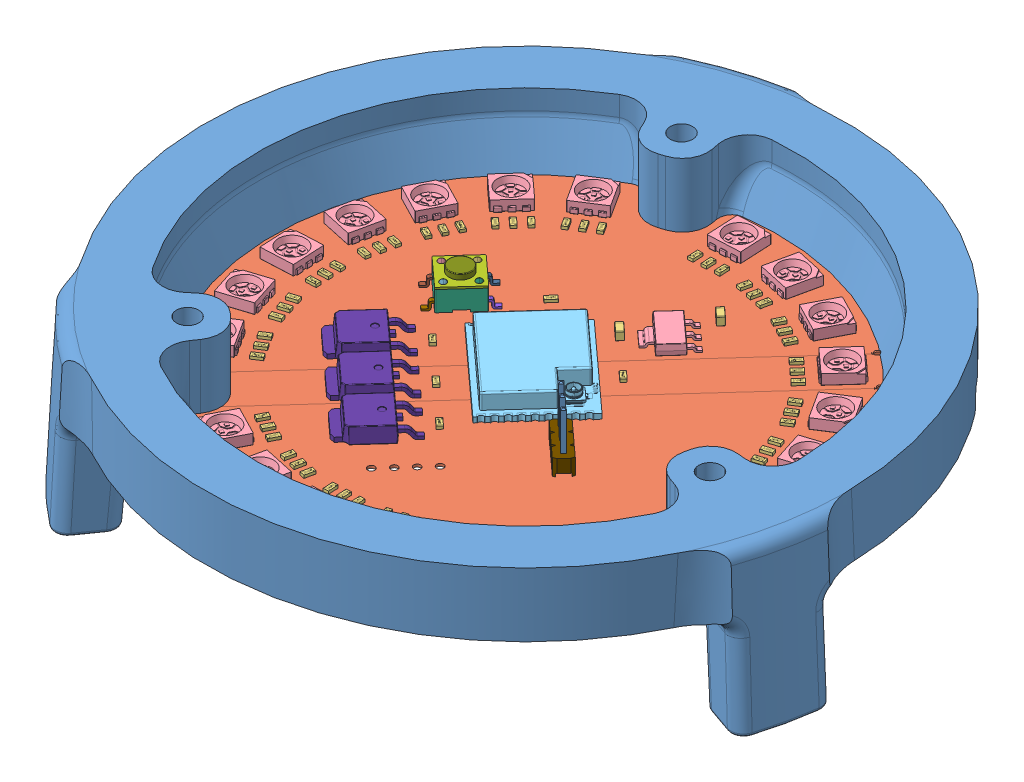
SolidWorks assembly Assem1, configuration Default. Lengths in mm.
Overall size (118.67 25.67 118.67).
223 component instances, 23 part files, 3 mates.
Components (placement in the parent):
- Part1-1: Part1 [Default] at (38.8159 57.1893 76.2452) size (102.81 25.67 101.93)
- PCB1.step-1: PCB1.step [Default] at (38.8159 57.1893 76.2451) x (-0.740561 0 -0.671989) z (0 1 0) size (84.01 84.01 11.86)
  - Board.step-1: Board.step [Default] at origin size (84.01 84.01 0.49)
    - Open CASCADE STEP translator 6.8 1.1.1.step-1: Open CASCADE STEP translator 6.8 1.1.1.step [Default] at (0 0 -0.4115) size (84.01 84.01 0.49)
  - R68.step-1: R68.step [Default] at origin size (1.6 0.8 0.45)
    - RES,0603.step-1: RES,0603.step [Default] at (-0.0001 -10.7188 0) x (-1 0 0) z (0 1 0) size (1.6 0.45 0.8)
  - U2.step-1: U2.step [Default] at origin size (6.5 6.96 1.68)
    - SOT223.step-1: SOT223.step [Default] at (7.1628 -16.2261 0.75) x (-1 0 0) z (0 1 0) size (6.5 1.68 6.96)
  - U1.step-1: U1.step [Default] at origin size (18.07 14.3 3.23)
    - ESP32-WROOM-02U.step-1: ESP32-WROOM-02U.step [Default] at (1.15 -0.85 0) x (-1 0 0) z (0 0 1) size (18.07 14.3 3.23)
  - SW1.step-1: SW1.step [Default] at origin size (6 9 4.3)
    - Switch,Tactile,SPST-NO,SMD.step-1: Switch,Tactile,SPST-NO,SMD.step [Default] at (16.4999 6.5001 0) x (0 1 0) z (0 0 1) size (9 6 4.3)
      - 1.step-1: 1.step [Default] at origin size (6 6 3.15)
      - 2.step-1: 2.step [Default] at origin size (6 6 0.3)
      - 3.step-1: 3.step [Default] at origin size (1.5 0.7 1.3)
      - 4.step-1: 4.step [Default] at origin size (1.5 0.7 1.3)
      - 5.step-1: 5.step [Default] at origin size (1.5 0.7 1.3)
      - 6.step-1: 6.step [Default] at origin size (1.5 0.7 1.3)
      - 7.step-1: 7.step [Default] at origin size (1 1 0.3)
      - 8.step-1: 8.step [Default] at origin size (1 1 0.3)
      - 9.step-1: 9.step [Default] at origin size (1 1 0.3)
      - 10.step-1: 10.step [Default] at origin size (1 1 0.3)
      - 11.step-1: 11.step [Default] at origin size (3.5 3.5 0.85)
  - R67.step-1: R67.step [Default] at origin size (1.6 0.8 0.45)
    - RES,0603.step-1: RES,0603.step [Default] at (-0.0001 10 0) x (-1 0 0) z (0 1 0) size (1.6 0.45 0.8)
  - R66.step-1: R66.step [Default] at origin size (0.8 1.6 0.45)
    - RES,0603.step-1: RES,0603.step [Default] at (15.23 -3.4601 0) x (0 -1 0) z (-1 0 0) size (1.6 0.45 0.8)
  - R65.step-1: R65.step [Default] at origin size (1.6 0.8 0.45)
    - RES,0603.step-1: RES,0603.step [Default] at (7.9999 10 0) x (-1 0 0) z (0 1 0) size (1.6 0.45 0.8)
  - R64.step-1: R64.step [Default] at origin size (1.6 0.8 0.45)
    - RES,0603.step-1: RES,0603.step [Default] at (-8.0001 10 0) x (-1 0 0) z (0 1 0) size (1.6 0.45 0.8)
  - R63.step-1: R63.step [Default] at origin size (1.19 1.75 0.45)
    - RES,0603.step-1: RES,0603.step [Default] at (9.6964 28.46 0) x (-0.258819 -0.965926 0) z (-0.965926 0.258819 0) size (1.6 0.45 0.8)
  - R62.step-1: R62.step [Default] at origin size (1.19 1.75 0.45)
    - RES,0603.step-1: RES,0603.step [Default] at (7.7646 28.9777 0) x (-0.258819 -0.965926 0) z (-0.965926 0.258819 0) size (1.6 0.45 0.8)
  - R61.step-1: R61.step [Default] at origin size (1.19 1.75 0.45)
    - RES,0603.step-1: RES,0603.step [Default] at (5.8327 29.4953 0) x (-0.258819 -0.965926 0) z (-0.965926 0.258819 0) size (1.6 0.45 0.8)
  - R60.step-1: R60.step [Default] at origin size (1.6 0.8 0.45)
    - RES,0603.step-1: RES,0603.step [Default] at (-29.9999 2 0) x (1 0 0) z (0 -1 0) size (1.6 0.45 0.8)
  - R59.step-1: R59.step [Default] at origin size (1.6 0.8 0.45)
    - RES,0603.step-1: RES,0603.step [Default] at (-29.9999 0 0) x (1 0 0) z (0 -1 0) size (1.6 0.45 0.8)
  - R58.step-1: R58.step [Default] at origin size (1.6 0.8 0.45)
    - RES,0603.step-1: RES,0603.step [Default] at (-29.9999 -2 0) x (1 0 0) z (0 -1 0) size (1.6 0.45 0.8)
  - R57.step-1: R57.step [Default] at origin size (1.7 1.7 0.45)
    - RES,0603.step-1: RES,0603.step [Default] at (22.6274 19.7989 0) x (-0.707107 -0.707107 0) z (-0.707107 0.707107 0) size (1.6 0.45 0.8)
  - R56.step-1: R56.step [Default] at origin size (1.7 1.7 0.45)
    - RES,0603.step-1: RES,0603.step [Default] at (21.2131 21.2131 0) x (-0.707107 -0.707107 0) z (-0.707107 0.707107 0) size (1.6 0.45 0.8)
  - R55.step-1: R55.step [Default] at origin size (1.7 1.7 0.45)
    - RES,0603.step-1: RES,0603.step [Default] at (19.7989 22.6273 0) x (-0.707107 -0.707107 0) z (-0.707107 0.707107 0) size (1.6 0.45 0.8)
  - R54.step-1: R54.step [Default] at origin size (1.75 1.19 0.45)
    - RES,0603.step-1: RES,0603.step [Default] at (-28.46 9.6964 0) x (0.965926 -0.258819 0) z (-0.258819 -0.965926 0) size (1.6 0.45 0.8)
  - R53.step-1: R53.step [Default] at origin size (1.75 1.19 0.45)
    - RES,0603.step-1: RES,0603.step [Default] at (-28.9777 7.7646 0) x (0.965926 -0.258819 0) z (-0.258819 -0.965926 0) size (1.6 0.45 0.8)
  - R52.step-1: R52.step [Default] at origin size (1.75 1.19 0.45)
    - RES,0603.step-1: RES,0603.step [Default] at (-29.4953 5.8327 0) x (0.965926 -0.258819 0) z (-0.258819 -0.965926 0) size (1.6 0.45 0.8)
  - R51.step-1: R51.step [Default] at origin size (1.49 1.79 0.45)
    - RES,0603.step-1: RES,0603.step [Default] at (-13.2679 26.9807 0) x (0.5 -0.866025 0) z (-0.866025 -0.5 0) size (1.6 0.45 0.8)
  - R50.step-1: R50.step [Default] at origin size (1.49 1.79 0.45)
    - RES,0603.step-1: RES,0603.step [Default] at (-14.9999 25.9807 0) x (0.5 -0.866025 0) z (-0.866025 -0.5 0) size (1.6 0.45 0.8)
  - R49.step-1: R49.step [Default] at origin size (1.49 1.79 0.45)
    - RES,0603.step-1: RES,0603.step [Default] at (-16.732 24.9807 0) x (0.5 -0.866025 0) z (-0.866025 -0.5 0) size (1.6 0.45 0.8)
  - R48.step-1: R48.step [Default] at origin size (1.6 0.8 0.45)
    - RES,0603.step-1: RES,0603.step [Default] at (29.9999 -2 0) x (-1 0 0) z (0 1 0) size (1.6 0.45 0.8)
  - R47.step-1: R47.step [Default] at origin size (1.6 0.8 0.45)
    - RES,0603.step-1: RES,0603.step [Default] at (29.9999 0 0) x (-1 0 0) z (0 1 0) size (1.6 0.45 0.8)
  - R46.step-1: R46.step [Default] at origin size (1.6 0.8 0.45)
    - RES,0603.step-1: RES,0603.step [Default] at (29.9999 2 0) x (-1 0 0) z (0 1 0) size (1.6 0.45 0.8)
  - R45.step-1: R45.step [Default] at origin size (1.49 1.79 0.45)
    - RES,0603.step-1: RES,0603.step [Default] at (16.732 24.9807 0) x (-0.5 -0.866025 0) z (-0.866025 0.5 0) size (1.6 0.45 0.8)
  - R44.step-1: R44.step [Default] at origin size (1.49 1.79 0.45)
    - RES,0603.step-1: RES,0603.step [Default] at (15 25.9806 0) x (-0.5 -0.866025 0) z (-0.866025 0.5 0) size (1.6 0.45 0.8)
  - R43.step-1: R43.step [Default] at origin size (1.49 1.79 0.45)
    - RES,0603.step-1: RES,0603.step [Default] at (13.2679 26.9807 0) x (-0.5 -0.866025 0) z (-0.866025 0.5 0) size (1.6 0.45 0.8)
  - R42.step-1: R42.step [Default] at origin size (1.19 1.75 0.45)
    - RES,0603.step-1: RES,0603.step [Default] at (-9.6964 -28.46 0) x (0.258819 0.965926 0) z (0.965926 -0.258819 0) size (1.6 0.45 0.8)
  - R41.step-1: R41.step [Default] at origin size (1.19 1.75 0.45)
    - RES,0603.step-1: RES,0603.step [Default] at (-7.7646 -28.9777 0) x (0.258819 0.965926 0) z (0.965926 -0.258819 0) size (1.6 0.45 0.8)
  - R40.step-1: R40.step [Default] at origin size (1.19 1.75 0.45)
    - RES,0603.step-1: RES,0603.step [Default] at (-5.8327 -29.4953 0) x (0.258819 0.965926 0) z (0.965926 -0.258819 0) size (1.6 0.45 0.8)
  - R39.step-1: R39.step [Default] at origin size (1.19 1.75 0.45)
    - RES,0603.step-1: RES,0603.step [Default] at (-5.8326 29.4953 0) x (0.258819 -0.965926 0) z (-0.965926 -0.258819 0) size (1.6 0.45 0.8)
  - R38.step-1: R38.step [Default] at origin size (1.19 1.75 0.45)
    - RES,0603.step-1: RES,0603.step [Default] at (-7.7645 28.9777 0) x (0.258819 -0.965926 0) z (-0.965926 -0.258819 0) size (1.6 0.45 0.8)
  - R37.step-1: R37.step [Default] at origin size (1.19 1.75 0.45)
    - RES,0603.step-1: RES,0603.step [Default] at (-9.6964 28.46 0) x (0.258819 -0.965926 0) z (-0.965926 -0.258819 0) size (1.6 0.45 0.8)
  - R36.step-1: R36.step [Default] at origin size (1.75 1.19 0.45)
    - RES,0603.step-1: RES,0603.step [Default] at (29.4953 5.8327 0) x (-0.965926 -0.258819 0) z (-0.258819 0.965926 0) size (1.6 0.45 0.8)
  - R35.step-1: R35.step [Default] at origin size (1.75 1.19 0.45)
    - RES,0603.step-1: RES,0603.step [Default] at (28.9777 7.7645 0) x (-0.965926 -0.258819 0) z (-0.258819 0.965926 0) size (1.6 0.45 0.8)
  - R34.step-1: R34.step [Default] at origin size (1.75 1.19 0.45)
    - RES,0603.step-1: RES,0603.step [Default] at (28.46 9.6964 0) x (-0.965926 -0.258819 0) z (-0.258819 0.965926 0) size (1.6 0.45 0.8)
  - R33.step-1: R33.step [Default] at origin size (1.75 1.19 0.45)
    - RES,0603.step-1: RES,0603.step [Default] at (28.46 -9.6964 0) x (-0.965926 0.258819 0) z (0.258819 0.965926 0) size (1.6 0.45 0.8)
  - R32.step-1: R32.step [Default] at origin size (1.75 1.19 0.45)
    - RES,0603.step-1: RES,0603.step [Default] at (28.9777 -7.7646 0) x (-0.965926 0.258819 0) z (0.258819 0.965926 0) size (1.6 0.45 0.8)
  - R31.step-1: R31.step [Default] at origin size (1.75 1.19 0.45)
    - RES,0603.step-1: RES,0603.step [Default] at (29.4953 -5.8327 0) x (-0.965926 0.258819 0) z (0.258819 0.965926 0) size (1.6 0.45 0.8)
  - R30.step-1: R30.step [Default] at origin size (1.7 1.7 0.45)
    - RES,0603.step-1: RES,0603.step [Default] at (-22.6274 -19.7989 0) x (0.707107 0.707107 0) z (0.707107 -0.707107 0) size (1.6 0.45 0.8)
  - R29.step-1: R29.step [Default] at origin size (1.7 1.7 0.45)
    - RES,0603.step-1: RES,0603.step [Default] at (-21.2132 -21.2131 0) x (0.707107 0.707107 0) z (0.707107 -0.707107 0) size (1.6 0.45 0.8)
  - R28.step-1: R28.step [Default] at origin size (1.7 1.7 0.45)
    - RES,0603.step-1: RES,0603.step [Default] at (-19.7989 -22.6273 0) x (0.707107 0.707107 0) z (0.707107 -0.707107 0) size (1.6 0.45 0.8)
  - R27.step-1: R27.step [Default] at origin size (0.8 1.6 0.45)
    - RES,0603.step-1: RES,0603.step [Default] at (-2 -29.9999 0) x (0 1 0) z (1 0 0) size (1.6 0.45 0.8)
  - R26.step-1: R26.step [Default] at origin size (0.8 1.6 0.45)
    - RES,0603.step-1: RES,0603.step [Default] at (0 -29.9999 0) x (0 1 0) z (1 0 0) size (1.6 0.45 0.8)
  - R25.step-1: R25.step [Default] at origin size (0.8 1.6 0.45)
    - RES,0603.step-1: RES,0603.step [Default] at (2 -29.9999 0) x (0 1 0) z (1 0 0) size (1.6 0.45 0.8)
  - R24.step-1: R24.step [Default] at origin size (1.19 1.75 0.45)
    - RES,0603.step-1: RES,0603.step [Default] at (5.8327 -29.4953 0) x (-0.258819 0.965926 0) z (0.965926 0.258819 0) size (1.6 0.45 0.8)
  - R23.step-1: R23.step [Default] at origin size (1.19 1.75 0.45)
    - RES,0603.step-1: RES,0603.step [Default] at (7.7645 -28.9777 0) x (-0.258819 0.965926 0) z (0.965926 0.258819 0) size (1.6 0.45 0.8)
  - R22.step-1: R22.step [Default] at origin size (1.19 1.75 0.45)
    - RES,0603.step-1: RES,0603.step [Default] at (9.6964 -28.46 0) x (-0.258819 0.965926 0) z (0.965926 0.258819 0) size (1.6 0.45 0.8)
  - R21.step-1: R21.step [Default] at origin size (1.79 1.49 0.45)
    - RES,0603.step-1: RES,0603.step [Default] at (-24.9807 16.732 0) x (0.866025 -0.5 0) z (-0.5 -0.866025 0) size (1.6 0.45 0.8)
  - R20.step-1: R20.step [Default] at origin size (1.79 1.49 0.45)
    - RES,0603.step-1: RES,0603.step [Default] at (-25.9807 15 0) x (0.866025 -0.5 0) z (-0.5 -0.866025 0) size (1.6 0.45 0.8)
  - R19.step-1: R19.step [Default] at origin size (1.79 1.49 0.45)
    - RES,0603.step-1: RES,0603.step [Default] at (-26.9806 13.2679 0) x (0.866025 -0.5 0) z (-0.5 -0.866025 0) size (1.6 0.45 0.8)
  - R18.step-1: R18.step [Default] at origin size (1.49 1.79 0.45)
    - RES,0603.step-1: RES,0603.step [Default] at (13.2679 -26.9807 0) x (-0.5 0.866025 0) z (0.866025 0.5 0) size (1.6 0.45 0.8)
  - R17.step-1: R17.step [Default] at origin size (1.49 1.79 0.45)
    - RES,0603.step-1: RES,0603.step [Default] at (14.9999 -25.9807 0) x (-0.5 0.866025 0) z (0.866025 0.5 0) size (1.6 0.45 0.8)
  - R16.step-1: R16.step [Default] at origin size (1.49 1.79 0.45)
    - RES,0603.step-1: RES,0603.step [Default] at (16.732 -24.9807 0) x (-0.5 0.866025 0) z (0.866025 0.5 0) size (1.6 0.45 0.8)
  - R15.step-1: R15.step [Default] at origin size (1.79 1.49 0.45)
    - RES,0603.step-1: RES,0603.step [Default] at (26.9807 13.2679 0) x (-0.866025 -0.5 0) z (-0.5 0.866025 0) size (1.6 0.45 0.8)
  - R14.step-1: R14.step [Default] at origin size (1.79 1.49 0.45)
    - RES,0603.step-1: RES,0603.step [Default] at (25.9807 14.9999 0) x (-0.866025 -0.5 0) z (-0.5 0.866025 0) size (1.6 0.45 0.8)
  - R13.step-1: R13.step [Default] at origin size (1.79 1.49 0.45)
    - RES,0603.step-1: RES,0603.step [Default] at (24.9807 16.732 0) x (-0.866025 -0.5 0) z (-0.5 0.866025 0) size (1.6 0.45 0.8)
  - R12.step-1: R12.step [Default] at origin size (1.7 1.7 0.45)
    - RES,0603.step-1: RES,0603.step [Default] at (19.7989 -22.6274 0) x (-0.707107 0.707107 0) z (0.707107 0.707107 0) size (1.6 0.45 0.8)
  - R11.step-1: R11.step [Default] at origin size (1.7 1.7 0.45)
    - RES,0603.step-1: RES,0603.step [Default] at (21.2131 -21.2132 0) x (-0.707107 0.707107 0) z (0.707107 0.707107 0) size (1.6 0.45 0.8)
  - R10.step-1: R10.step [Default] at origin size (1.7 1.7 0.45)
    - RES,0603.step-1: RES,0603.step [Default] at (22.6273 -19.799 0) x (-0.707107 0.707107 0) z (0.707107 0.707107 0) size (1.6 0.45 0.8)
  - R9.step-1: R9.step [Default] at origin size (1.49 1.79 0.45)
    - RES,0603.step-1: RES,0603.step [Default] at (-16.732 -24.9807 0) x (0.5 0.866025 0) z (0.866025 -0.5 0) size (1.6 0.45 0.8)
  - R8.step-1: R8.step [Default] at origin size (1.49 1.79 0.45)
    - RES,0603.step-1: RES,0603.step [Default] at (-15 -25.9806 0) x (0.5 0.866025 0) z (0.866025 -0.5 0) size (1.6 0.45 0.8)
  - R7.step-1: R7.step [Default] at origin size (1.49 1.79 0.45)
    - RES,0603.step-1: RES,0603.step [Default] at (-13.2679 -26.9806 0) x (0.5 0.866025 0) z (0.866025 -0.5 0) size (1.6 0.45 0.8)
  - R6.step-1: R6.step [Default] at origin size (1.7 1.7 0.45)
    - RES,0603.step-1: RES,0603.step [Default] at (-19.7989 22.6274 0) x (0.707107 -0.707107 0) z (-0.707107 -0.707107 0) size (1.6 0.45 0.8)
  - R5.step-1: R5.step [Default] at origin size (1.7 1.7 0.45)
    - RES,0603.step-1: RES,0603.step [Default] at (-21.2131 21.2132 0) x (0.707107 -0.707107 0) z (-0.707107 -0.707107 0) size (1.6 0.45 0.8)
  - R4.step-1: R4.step [Default] at origin size (1.7 1.7 0.45)
    - RES,0603.step-1: RES,0603.step [Default] at (-22.6273 19.7989 0) x (0.707107 -0.707107 0) z (-0.707107 -0.707107 0) size (1.6 0.45 0.8)
  - R3.step-1: R3.step [Default] at origin size (1.75 1.19 0.45)
    - RES,0603.step-1: RES,0603.step [Default] at (-29.4953 -5.8326 0) x (0.965926 0.258819 0) z (0.258819 -0.965926 0) size (1.6 0.45 0.8)
  - R2.step-1: R2.step [Default] at origin size (1.75 1.19 0.45)
    - RES,0603.step-1: RES,0603.step [Default] at (-28.9777 -7.7645 0) x (0.965926 0.258819 0) z (0.258819 -0.965926 0) size (1.6 0.45 0.8)
  - R1.step-1: R1.step [Default] at origin size (1.75 1.19 0.45)
    - RES,0603.step-1: RES,0603.step [Default] at (-28.46 -9.6964 0) x (0.965926 0.258819 0) z (0.258819 -0.965926 0) size (1.6 0.45 0.8)
  - Q3.step-1: Q3.step [Default] at origin size (6.72 10.41 2.39)
    - TO-252.step-1: TO-252.step [Default] at (0.0001 17 0) x (1 0 0) z (0 0 1) size (6.72 10.41 2.39)
      - Open CASCADE STEP translator 6.8 1.73.1.1.step-1: Open CASCADE STEP translator 6.8 1.73.1.1.step [Default] at origin size (6.72 10.41 2.39)
      - Open CASCADE STEP translator 6.8 1.73.1.2.step-1: Open CASCADE STEP translator 6.8 1.73.1.2.step [Default] at origin
  - Q2.step-1: Q2.step [Default] at origin size (6.72 10.41 2.39)
    - TO-252.step-1: TO-252.step [Default] at (8.0001 17 0) x (1 0 0) z (0 0 1) size (6.72 10.41 2.39)
      - Open CASCADE STEP translator 6.8 1.73.1.1.step-1: Open CASCADE STEP translator 6.8 1.73.1.1.step [Default] at origin size (6.72 10.41 2.39)
      - Open CASCADE STEP translator 6.8 1.73.1.2.step-1: Open CASCADE STEP translator 6.8 1.73.1.2.step [Default] at origin
  - Q1.step-1: Q1.step [Default] at origin size (6.72 10.41 2.39)
    - TO-252.step-1: TO-252.step [Default] at (-7.9999 17 0) x (1 0 0) z (0 0 1) size (6.72 10.41 2.39)
      - Open CASCADE STEP translator 6.8 1.73.1.1.step-1: Open CASCADE STEP translator 6.8 1.73.1.1.step [Default] at origin size (6.72 10.41 2.39)
      - Open CASCADE STEP translator 6.8 1.73.1.2.step-1: Open CASCADE STEP translator 6.8 1.73.1.2.step [Default] at origin
  - J6.step-1: J6.step [Default] at origin size (7.62 2.54 11.54)
    - Term,Header,3Pin,2.54mm.step-1: Term,Header,3Pin,2.54mm.step [Default] at (-14.8589 -3.2511 1.3) x (1 0 0) z (0 -1 0) size (7.62 11.54 2.54)
      - 61300311121.step-1: 61300311121.step [Default] at origin size (7.62 2.54 2.54)
      - 6130xx11121_PIN.step-1: 6130xx11121_PIN.step [Default] at (-2.54 1.5 0) x (1 0 0) z (0 -1 0) size (0.64 0.64 11.54)
      - 6130xx11121_PIN.step-2: 6130xx11121_PIN.step [Default] at (0 1.5 0) x (1 0 0) z (0 -1 0) size (0.64 0.64 11.54)
      - 6130xx11121_PIN.step-3: 6130xx11121_PIN.step [Default] at (2.54 1.5 0) x (1 0 0) z (0 -1 0) size (0.64 0.64 11.54)
  - J1.step-1: J1.step [Default] at origin size (7.87 5.71 3.61)
    - Conn,USB,MicroB,SMD.step-1: Conn,USB,MicroB,SMD.step [Default] at (98.0119 -35.9065 -0.1115) x (-1 0 0) z (0 -1 0) size (7.87 3.61 5.71)
  - C2.step-1: C2.step [Default] at origin size (2 1 1.2)
    - CAP,SMD,0805.step-1: CAP,SMD,0805.step [Default] at (8.1627 -11.2188 0.6) x (-1 0 0) z (0 1 0) size (2 1.2 1)
  - C1.step-1: C1.step [Default] at origin size (2 1 1.2)
    - CAP,SMD,0805.step-1: CAP,SMD,0805.step [Default] at (10.4627 -22.5 0.6) x (-1 0 0) z (0 1 0) size (2 1.2 1)
  - D9.step-1: D9.step [Default] at origin size (5 5.4 1.62)
    - LED_SMD_5050_RGB.step-1: LED_SMD_5050_RGB.step [Default] at (-1.6 -37.2 0) x (0 1 0) z (0 0 1) size (5.4 5 1.62)
  - D13.step-1: D13.step [Default] at origin size (6.23 6.51 1.62)
    - LED_SMD_5050_RGB.step-1: LED_SMD_5050_RGB.step [Default] at (-8.0826 36.3465 0) x (0.258819 -0.965926 0) z (0 0 1) size (5.4 5 1.62)
  - D3.step-1: D3.step [Default] at origin size (7.03 7.18 1.62)
    - LED_SMD_5050_RGB.step-1: LED_SMD_5050_RGB.step [Default] at (-19.9856 -31.4161 0) x (0.5 0.866025 0) z (0 0 1) size (5.4 5 1.62)
  - D21.step-1: D21.step [Default] at origin size (6.23 6.51 1.62)
    - LED_SMD_5050_RGB.step-1: LED_SMD_5050_RGB.step [Default] at (11.1735 35.5183 0) x (-0.258819 -0.965926 0) z (0 0 1) size (5.4 5 1.62)
  - D8.step-1: D8.step [Default] at origin size (6.23 6.51 1.62)
    - LED_SMD_5050_RGB.step-1: LED_SMD_5050_RGB.step [Default] at (8.0826 -36.3465 0) x (-0.258819 0.965926 0) z (0 0 1) size (5.4 5 1.62)
  - D6.step-1: D6.step [Default] at origin size (7.03 7.18 1.62)
    - LED_SMD_5050_RGB.step-1: LED_SMD_5050_RGB.step [Default] at (17.2143 -33.0161 0) x (-0.5 0.866025 0) z (0 0 1) size (5.4 5 1.62)
  - D5.step-1: D5.step [Default] at origin size (7.18 7.03 1.62)
    - LED_SMD_5050_RGB.step-1: LED_SMD_5050_RGB.step [Default] at (33.0161 17.2143 0) x (-0.866025 -0.5 0) z (0 0 1) size (5.4 5 1.62)
  - D14.step-1: D14.step [Default] at origin size (6.23 6.51 1.62)
    - LED_SMD_5050_RGB.step-1: LED_SMD_5050_RGB.step [Default] at (-11.1735 -35.5183 0) x (0.258819 0.965926 0) z (0 0 1) size (5.4 5 1.62)
  - D19.step-1: D19.step [Default] at origin size (7.35 7.35 1.62)
    - LED_SMD_5050_RGB.step-1: LED_SMD_5050_RGB.step [Default] at (27.4357 25.173 0) x (-0.707107 -0.707107 0) z (0 0 1) size (5.4 5 1.62)
  - D15.step-1: D15.step [Default] at origin size (7.03 7.18 1.62)
    - LED_SMD_5050_RGB.step-1: LED_SMD_5050_RGB.step [Default] at (19.9856 31.4161 0) x (-0.5 -0.866025 0) z (0 0 1) size (5.4 5 1.62)
  - D2.step-1: D2.step [Default] at origin size (7.35 7.35 1.62)
    - LED_SMD_5050_RGB.step-1: LED_SMD_5050_RGB.step [Default] at (-25.173 27.4357 0) x (0.707107 -0.707107 0) z (0 0 1) size (5.4 5 1.62)
  - D16.step-1: D16.step [Default] at origin size (5.4 5 1.62)
    - LED_SMD_5050_RGB.step-1: LED_SMD_5050_RGB.step [Default] at (37.2 -1.6 0) x (-1 0 0) z (0 0 1) size (5.4 5 1.62)
  - D4.step-1: D4.step [Default] at origin size (7.35 7.35 1.62)
    - LED_SMD_5050_RGB.step-1: LED_SMD_5050_RGB.step [Default] at (25.173 -27.4357 0) x (-0.707107 0.707107 0) z (0 0 1) size (5.4 5 1.62)
  - D10.step-1: D10.step [Default] at origin size (7.35 7.35 1.62)
    - LED_SMD_5050_RGB.step-1: LED_SMD_5050_RGB.step [Default] at (-27.4357 -25.173 0) x (0.707107 0.707107 0) z (0 0 1) size (5.4 5 1.62)
  - D20.step-1: D20.step [Default] at origin size (5.4 5 1.62)
    - LED_SMD_5050_RGB.step-1: LED_SMD_5050_RGB.step [Default] at (-37.2 1.6 0) x (1 0 0) z (0 0 1) size (5.4 5 1.62)
  - D11.step-1: D11.step [Default] at origin size (6.51 6.23 1.62)
    - LED_SMD_5050_RGB.step-1: LED_SMD_5050_RGB.step [Default] at (35.5183 -11.1735 0) x (-0.965926 0.258819 0) z (0 0 1) size (5.4 5 1.62)
  - D12.step-1: D12.step [Default] at origin size (6.51 6.23 1.62)
    - LED_SMD_5050_RGB.step-1: LED_SMD_5050_RGB.step [Default] at (36.3465 8.0826 0) x (-0.965926 -0.258819 0) z (0 0 1) size (5.4 5 1.62)
  - D7.step-1: D7.step [Default] at origin size (7.18 7.03 1.62)
    - LED_SMD_5050_RGB.step-1: LED_SMD_5050_RGB.step [Default] at (-31.4161 19.9856 0) x (0.866025 -0.5 0) z (0 0 1) size (5.4 5 1.62)
  - D18.step-1: D18.step [Default] at origin size (6.51 6.23 1.62)
    - LED_SMD_5050_RGB.step-1: LED_SMD_5050_RGB.step [Default] at (-35.5183 11.1735 0) x (0.965926 -0.258819 0) z (0 0 1) size (5.4 5 1.62)
  - D1.step-1: D1.step [Default] at origin size (6.51 6.23 1.62)
    - LED_SMD_5050_RGB.step-1: LED_SMD_5050_RGB.step [Default] at (-36.3465 -8.0826 0) x (0.965926 0.258819 0) z (0 0 1) size (5.4 5 1.62)
  - D17.step-1: D17.step [Default] at origin size (7.03 7.18 1.62)
    - LED_SMD_5050_RGB.step-1: LED_SMD_5050_RGB.step [Default] at (-17.2143 33.0161 0) x (0.5 -0.866025 0) z (0 0 1) size (5.4 5 1.62)
Mates (geometry in assembly coordinates):
- Coincident1: coincident anti-aligned: plane of Part1-1 through (38.8159 57.1893 76.2452) normal (0 -1 0); plane of PCB1.step-1/Board.step-1/Open CASCADE STEP translator 6.8 1.1.1.step-1 through (8.085 57.1893 48.2912) normal (0 1 0)
- Concentric1: concentric anti-aligned: cylinder of Part1-1 through (75.4661 57.1893 84.1831) axis (0 1 0) radius 1.75; cylinder of PCB1.step-1/Board.step-1/Open CASCADE STEP translator 6.8 1.1.1.step-1 through (75.466 56.7778 84.1831) axis (0 -1 0) radius 1.75
- Concentric2: concentric anti-aligned: cylinder of Part1-1 through (27.3652 57.1893 40.5362) axis (0 1 0) radius 1.75; cylinder of PCB1.step-1/Board.step-1/Open CASCADE STEP translator 6.8 1.1.1.step-1 through (27.3652 56.7778 40.5362) axis (0 -1 0) radius 1.75
